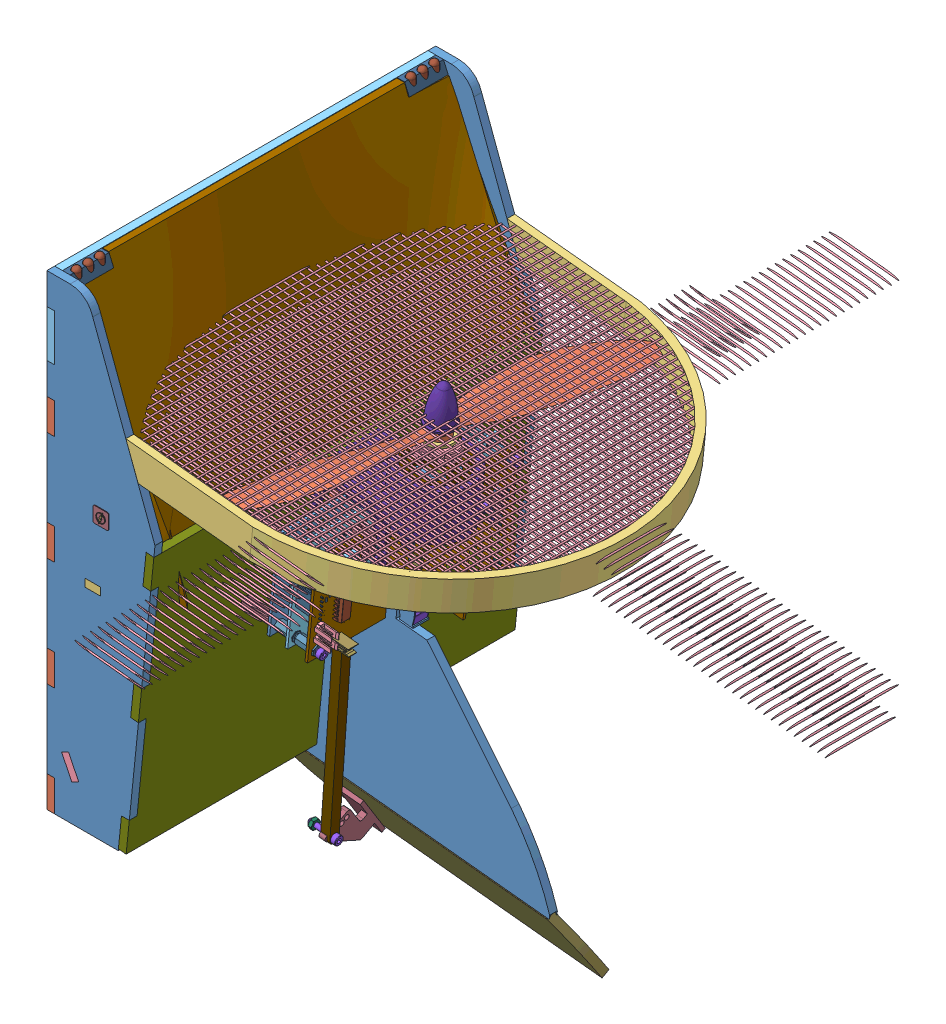
SolidWorks assembly AssTotaleSimu4, configuration Défaut. Lengths in mm. (continued)
Components (placement in the parent): (continued)
- AssStructSimu-1: AssStructSimu [Défaut] at (-125.7658 -1.8483 624.6548) x (1 0 0) z (0 0 -1) size (253.25 324.59 251.6) (continued)
  - AssCarte-1: AssCarte [Défaut] at (38.0121 147.1029 290.772) x (-0.101852 0.9948 0) z (0.9948 0.101852 0) size (66.52 130.57 98.72) (continued)
    - AssEntretoise-3: AssEntretoise [Défaut] at (-106.8199 -51.2976 37.1344) x (0 0 -1) z (1 0 0) size (58.24 7.29 7.81)
      - socket head cap screw 4762_din-1: socket head cap screw 4762_din [EN ISO 4762 M3 x 5 - 5N] at (-2.4967 0.5867 0) size (8 5.5 5.5)
      - hexagonal_spacer_MF_M3_H20_HEX5.5_FTD6_MTL6-1: hexagonal_spacer_MF_M3_H20_HEX5.5_FTD6_MTL6 [Défaut] at (48.3433 0.5867 0) x (0 0 1) z (-1 0 0) size (6.36 5.51 26)
      - hex nut style 1 gradeab_din-1: hex nut style 1 gradeab_din [Hexagon Nut ISO 4032 - M3 - W - N] at (53.3433 0.5867 0) x (0 0.943962 0.330053) z (-1 0 0) size (5.5 6.35 2.4)
      - hexagonal_spacer_MF_M3_H12_HEX5.5_FTD6_MTL6-2: hexagonal_spacer_MF_M3_H12_HEX5.5_FTD6_MTL6 [Défaut] at (27.0633 0.5867 0) x (0 0.248308 0.968681) z (-1 0 0) size (6.36 5.51 18)
      - hexagonal_spacer_MF_M3_H12_HEX5.5_FTD6_MTL6-3: hexagonal_spacer_MF_M3_H12_HEX5.5_FTD6_MTL6 [Défaut] at (13.7833 0.5867 0) x (0 0 1) z (-1 0 0) size (6.36 5.51 18)
    - AssEntretoise-4: AssEntretoise [Défaut] at (-106.8199 68.7024 37.1344) x (0 0 -1) z (1 0 0) size (58.24 7.29 7.81)
      - socket head cap screw 4762_din-1: socket head cap screw 4762_din [EN ISO 4762 M3 x 5 - 5N] at (-2.4967 0.5867 0) size (8 5.5 5.5)
      - hexagonal_spacer_MF_M3_H20_HEX5.5_FTD6_MTL6-1: hexagonal_spacer_MF_M3_H20_HEX5.5_FTD6_MTL6 [Défaut] at (48.3433 0.5867 0) x (0 0 1) z (-1 0 0) size (6.36 5.51 26)
      - hex nut style 1 gradeab_din-1: hex nut style 1 gradeab_din [Hexagon Nut ISO 4032 - M3 - W - N] at (53.3433 0.5867 0) x (0 0.943962 0.330053) z (-1 0 0) size (5.5 6.35 2.4)
      - hexagonal_spacer_MF_M3_H12_HEX5.5_FTD6_MTL6-2: hexagonal_spacer_MF_M3_H12_HEX5.5_FTD6_MTL6 [Défaut] at (27.0633 0.5867 0) x (0 0.248308 0.968681) z (-1 0 0) size (6.36 5.51 18)
      - hexagonal_spacer_MF_M3_H12_HEX5.5_FTD6_MTL6-3: hexagonal_spacer_MF_M3_H12_HEX5.5_FTD6_MTL6 [Défaut] at (13.7833 0.5867 0) x (0 0 1) z (-1 0 0) size (6.36 5.51 18)
    - AssMpu-1: AssMpu [Défaut] at (-150.6881 40.5798 29.6372) x (0.908747 0.417347 0) z (0 0 1) size (8 8 22.28)
      - hex nut style 1 gradeab_din-1: hex nut style 1 gradeab_din [Hexagon Nut ISO 4032 - M3 - W - N] at (0.2783 0.3227 1.2) size (5.5 6.35 2.4)
      - plain washer 6903 type ab_din-1: plain washer 6903 type ab_din [DIN 6903-A3] at (0.2783 0.3227 1.2) x (0 0 1) z (-1 0 0) size (1 8 8)
      - socket head cap screw 4762_din-1: socket head cap screw 4762_din [EN ISO 4762 M3 x 5 - 5N] at (0.2783 0.3227 19.76) x (0 0 -1) z (-0.852155 0.523289 0) size (8 5.5 5.5)
      - hexagonal_spacer_MF_M3_H12_HEX5.5_FTD6_MTL6-1: hexagonal_spacer_MF_M3_H12_HEX5.5_FTD6_MTL6 [Défaut] at (0.2783 0.3227 3.48) size (6.36 5.51 18)
    - AssMpu-2: AssMpu [Défaut] at (-130.3481 40.6665 29.6372) size (8 8 22.28)
      - hex nut style 1 gradeab_din-1: hex nut style 1 gradeab_din [Hexagon Nut ISO 4032 - M3 - W - N] at (0.2783 0.3227 1.2) size (5.5 6.35 2.4)
      - plain washer 6903 type ab_din-1: plain washer 6903 type ab_din [DIN 6903-A3] at (0.2783 0.3227 1.2) x (0 0 1) z (-1 0 0) size (1 8 8)
      - socket head cap screw 4762_din-1: socket head cap screw 4762_din [EN ISO 4762 M3 x 5 - 5N] at (0.2783 0.3227 19.76) x (0 0 -1) z (-0.852155 0.523289 0) size (8 5.5 5.5)
      - hexagonal_spacer_MF_M3_H12_HEX5.5_FTD6_MTL6-1: hexagonal_spacer_MF_M3_H12_HEX5.5_FTD6_MTL6 [Défaut] at (0.2783 0.3227 3.48) size (6.36 5.51 18)
    - AssCosse-1: AssCosse [Défaut] at (-142.6764 26.8797 71.168) x (0 -1 0) z (-0.344896 0 -0.938641) size (9.83 18.66 11.64)
      - socket head cap screw 4762_din-1: socket head cap screw 4762_din [EN ISO 4762 M3 x 6 - 6N] at (-5.1064 0.3659 0) size (9 5.5 5.5)
      - plain washer 6903 type ab_din-1: plain washer 6903 type ab_din [DIN 6903-A3] at (-2.1064 0.3659 0) size (1 8 8)
      - hex nut style 1 gradeab_din-2: hex nut style 1 gradeab_din [Hexagon Nut ISO 4032 - M3 - W - N] at (1.281 0.3659 0) x (0 0.924225 0.381849) z (-1 0 0) size (5.5 6.35 2.4)
      - 31880-1: 31880 [Default] at (0.4936 0.3659 0) x (0 0.344896 -0.938641) z (0 -0.938641 -0.344896) size (5.54 5 17.37)
    - AssCosse-2: AssCosse [Défaut] at (-142.6764 -2.9203 71.168) x (0 -1 0) z (-0.344896 0 -0.938641) size (9.83 18.66 11.64)
      - socket head cap screw 4762_din-1: socket head cap screw 4762_din [EN ISO 4762 M3 x 6 - 6N] at (-5.1064 0.3659 0) size (9 5.5 5.5)
      - plain washer 6903 type ab_din-1: plain washer 6903 type ab_din [DIN 6903-A3] at (-2.1064 0.3659 0) size (1 8 8)
      - hex nut style 1 gradeab_din-2: hex nut style 1 gradeab_din [Hexagon Nut ISO 4032 - M3 - W - N] at (1.281 0.3659 0) x (0 0.924225 0.381849) z (-1 0 0) size (5.5 6.35 2.4)
      - 31880-1: 31880 [Default] at (0.4936 0.3659 0) x (0 0.344896 -0.938641) z (0 -0.938641 -0.344896) size (5.54 5 17.37)
    - AssCosse-3: AssCosse [Défaut] at (-142.6764 12.0797 71.168) x (0 -1 0) z (-0.344896 0 -0.938641) size (9.83 18.66 11.64)
      - socket head cap screw 4762_din-1: socket head cap screw 4762_din [EN ISO 4762 M3 x 6 - 6N] at (-5.1064 0.3659 0) size (9 5.5 5.5)
      - plain washer 6903 type ab_din-1: plain washer 6903 type ab_din [DIN 6903-A3] at (-2.1064 0.3659 0) size (1 8 8)
      - hex nut style 1 gradeab_din-2: hex nut style 1 gradeab_din [Hexagon Nut ISO 4032 - M3 - W - N] at (1.281 0.3659 0) x (0 0.924225 0.381849) z (-1 0 0) size (5.5 6.35 2.4)
      - 31880-1: 31880 [Default] at (0.4936 0.3659 0) x (0 0.344896 -0.938641) z (0 -0.938641 -0.344896) size (5.54 5 17.37)
    - Terminal_QD_Female-1: Terminal_QD_Female [Default] at (-137.2199 31.5422 53.3942) x (0 1 0) z (-1 0 0) size (9.4 5.5 22.35)
    - Terminal_QD_Female-2: Terminal_QD_Female [Default] at (-137.3199 31.5422 36.2942) x (0 -1 0) z (-1 0 0) size (9.4 5.5 22.35)
    - Terminal_QD_Female-3: Terminal_QD_Female [Default] at (-137.2199 1.7422 53.3942) x (0 1 0) z (-1 0 0) size (9.4 5.5 22.35)
    - Terminal_QD_Female-4: Terminal_QD_Female [Default] at (-137.3199 1.7422 35.9942) x (0 1 0) z (-1 0 0) size (9.4 5.5 22.35)
    - Terminal_QD_Female-5: Terminal_QD_Female [Default] at (-137.3199 16.7422 35.9942) x (0 1 0) z (-1 0 0) size (9.4 5.5 22.35)
    - Terminal_QD_Female-6: Terminal_QD_Female [Default] at (-137.2199 16.7422 53.3942) x (0 1 0) z (-1 0 0) size (9.4 5.5 22.35)
- AssTige-1: AssTige [Défaut] at (-241.576 -121.7726 340.4233) x (-0.101791 -0.994204 -0.034587) z (0.9948 -0.101852 0) size (166.39 7.19 19)
  - tige_servo-1: tige_servo [Défaut] at (-106.2712 0.2685 162) size (165 6 6)
  - socket head cap screw 4762_din-2: socket head cap screw 4762_din [EN ISO 4762 M2 x 10 - 10N] at (-104.2712 3.2685 170) x (0 0 -1) z (0.923728 0.383049 0) size (12 3.8 3.8)
  - hex nut style 1 gradeab_din-1: hex nut style 1 gradeab_din [Hexagon Nut ISO 4032 - M3 - W - N] at (55.7288 3.2685 156) size (5.5 6.35 2.4)
  - hex nut style 1 gradeab_din-2: hex nut style 1 gradeab_din [Hexagon Nut ISO 4032 - M2 - W - N] at (-104.2712 3.2685 160) x (0.904801 0.425836 0) z (0 0 1) size (4 4.62 1.6)
  - socket head cap screw 4762_din-3: socket head cap screw 4762_din [EN ISO 4762 M3 x 16 - 16N] at (55.7288 3.2685 171) x (0 0 -1) z (0.923728 0.383049 0) size (19 5.5 5.5)
- AssGoPro-1: AssGoPro [Défaut] at (-119.9926 15.1708 318.2917) x (0 0 -1) z (-0.119031 -0.99289 0) size (64.3 52.3 34.42)
  - GoPRo Frame for LCD Screen-1: GoPRo Frame for LCD Screen [Défaut] at (-2.6935 10.9558 5.5635) size (64.3 59.3 34.42)
    - GoProFrame MJM-1: GoProFrame MJM [Défaut] at (-3.6084 -1.6692 52.45) size (64.3 59.3 23.5)
    - GoPro Hero 3 Front Panel-1: GoPro Hero 3 Front Panel [Défaut] at (-3.6084 -1.6692 55.7) x (-1 0 0) z (0 0 -1) size (59.25 41.2 1.9)
    - GoPro Hero 3 Screen-1: GoPro Hero 3 Screen [Défaut] at (12.7166 3.9308 54.9) size (15 18 1)
    - GoPro Hero 3 Mode Button-1: GoPro Hero 3 Mode Button [Défaut] at (13.4166 -12.4692 54.95) x (-1 0 0) z (0 0 -1) size (11.97 12.11 3.03)
    - GoPro Hero 3 LED Cover-1: GoPro Hero 3 LED Cover [Défaut] at (3.1166 -9.3192 54.85) x (-0.999988 0.004848 0) z (0 0 -1) size (5 5 1.4)
    - GoPro Hero 3 LED Cover-2: GoPro Hero 3 LED Cover [Défaut] at (3.1166 -16.0692 54.85) x (-0.999988 0.004848 0) z (0 0 -1) size (5 5 1.4)
    - GoPro Hero 3 Housing-1: GoPro Hero 3 Housing [Défaut] at (-3.6084 -1.6692 55.7) size (59.37 41.3 29.84)
    - GoPro Hero 3 Lens-1: GoPro Hero 3 Lens [Défaut] at (-18.9334 5.6308 47.35) x (-0.380542 -0.924764 0) z (0 0 -1) size (13.71 15.7 7.94)
    - GoPro Hero 3 Indicator Cover-1: GoPro Hero 3 Indicator Cover [Défaut] at (-25.5834 -22.2692 69.9) x (-0.997412 0 -0.0719) z (0 1 0) size (3 3 2)
    - GoPro Hero 3 Indicator Cover-2: GoPro Hero 3 Indicator Cover [Défaut] at (-28.8834 12.2308 73) x (-0.999992 0.004018 0) z (0 0 1) size (3 3 2)
    - GoPro Hero 3 Indicator Cover-3: GoPro Hero 3 Indicator Cover [Défaut] at (20.6666 16.9308 58.4) x (-0.997739 0 -0.067212) z (0 1 0) size (3 3 2)
    - slot-1: slot [Défaut] at (-24.7434 -9.7363 65.05) x (0 1 0) z (0 0 -1) size (16 15.02 2.44)
    - GoPro Hero 3 HDMI pin-1: GoPro Hero 3 HDMI pin [Défaut] at (-26.982 2.9815 24.7172) x (0.105491 0.98175 -0.158237) z (-0.992872 0.095109 -0.071829) size (3.29 0.86 3.28)
  - support1-2: support1 [Défaut] at (-1.3019 -18.8633 67.0135) x (0 0 1) z (-1 0 0) size (5 5 10)
- AssGouv-1: AssGouv [Défaut] at (-43.2668 -298.2106 479.8345) x (0.9948 -0.101852 0) z (0.055947 0.546439 -0.835628) size (200.18 52.5 43.47)
  - P10_1-1: P10_1 [Défaut] at (-108.1667 -19.4144 197.6829) size (200.18 50.13 5)
  - attache_pale-1: attache_pale [Défaut] at (-49.1667 8.0856 190.1829) x (0 0 -1) z (-1 0 0) size (43.47 35 14)
- Parallax-Servo-Horn-1: Parallax-Servo-Horn [Défaut] at (-69.3162 -29.8353 324.5606) x (0.09792 0.956393 0.27518) z (0.9948 -0.101852 0) size (38.81 38.81 6.17)
- NTM_35-36_engine_assembly-1: NTM_35-36_engine_assembly [Défaut] at (-24.3523 26.8781 325.7101) x (0.9948 -0.101852 0) z (0 0 1) size (60.56 77.2 246.41)
  - engine_base-1: engine_base [Défaut] at (-1.8719 -19.5526 -1.1165) x (0 1 0) z (0 0 1) size (6.8 35 35)
  - engine_bearing-1: engine_bearing [Défaut] at origin size (10 4 10)
  - Propeller_cone-1: Propeller_cone [Défaut] at (-1.8719 33.6474 -4.1165) x (1 0 0) z (0 1 0) size (17.6 17.6 24)
  - engine_bearing-2: engine_bearing [Défaut] at (0 22.8 0) size (10 4 10)
  - NTM_35-36_enginebody-1: NTM_35-36_enginebody [Défaut] at (-1.8719 -12.7526 -1.1165) size (35 31.7 35)
  - Stator-1: Stator [Défaut] at origin size (27.75 22.36 27.94)
  - propellers_10x4-1: propellers_10x4 [Défaut] at (-6.8719 27.4474 -4.9165) size (60.56 10.53 246.41)
  - propeller_washer-1: propeller_washer [Défaut] at (-1.8719 24.4474 -1.1165) x (0 1 0) z (0 0 1) size (2.5 18 18)
  - Propeller_adaptor-1: Propeller_adaptor [Défaut] at (2.1948 17.1101 -3.713) size (23.46 32.5 25)
Mates (geometry in assembly coordinates):
- Coaxiale1: concentric aligned: cylinder of AssStructSimu-1/AssToitMot-1/AssToit-1/P12-1 through (-27.6967 12.5918 324.5936) axis (-0.101852 -0.9948 0) radius 17.5; cylinder of NTM_35-36_engine_assembly-1/NTM_35-36_enginebody-1 through (-25.2217 36.7654 324.5936) axis (-0.101852 -0.9948 0) radius 17.5
- Coïncidente1: coincident anti-aligned: plane of AssStructSimu-1/AssToitMot-1/AssToit-1/P12-1 through (-28.206 7.6178 324.5936) normal (0.101852 0.9948 0); plane of NTM_35-36_engine_assembly-1/engine_bearing-1 through (-28.206 7.6178 324.5936) normal (-0.101852 -0.9948 0)
- Coaxiale2: concentric aligned: cylinder of AssStructSimu-1/AssToitMot-1/AssToit-1/P10_2-1 through (49.7135 -178.7878 324.5936) axis (-0.9948 0.101852 0) radius 2.5; cylinder of AssGouv-1/P10_1-1 through (-94.0351 -164.0702 324.5936) axis (-0.9948 0.101852 0) radius 2.5
- Coïncidente2: coincident aligned: plane of AssStructSimu-1/AssToitMot-1/AssToit-1/P10_2-1 through (-137.5516 -157.1017 322.0936) normal (-0.9948 0.101852 0); plane of AssGouv-1/P10_1-1 through (-137.8791 -160.3008 321.1312) normal (-0.9948 0.101852 0)
- Coaxiale3: concentric aligned: cylinder of AssTige-1/socket head cap screw 4762_din-3 through (-45.5416 -197.7164 335.2292) axis (0.9948 -0.101852 0) radius 1.5; cylinder of AssGouv-1/attache_pale-1 through (-85.9983 -193.5742 335.2292) axis (0.9948 -0.101852 0) radius 1.5
- Coaxiale4: concentric aligned: cylinder of AssStructSimu-1/AssToitMot-1/Parallax-Servo_DUMMY-1 through (-70.6554 -29.6982 324.5606) axis (-0.9948 0.101852 0) radius 2.9845; cylinder of Parallax-Servo-Horn-1 through (-70.6554 -29.6982 324.5606) axis (-0.9948 0.101852 0) radius 2.9845
- Coïncidente3: coincident anti-aligned: plane of AssStructSimu-1/AssToitMot-1/Parallax-Servo_DUMMY-1 through (-74.8246 -29.2713 324.5606) normal (0.9948 -0.101852 0); plane of Parallax-Servo-Horn-1 through (-74.8246 -29.2713 324.5606) normal (-0.9948 0.101852 0)
- Coaxiale5: concentric anti-aligned: cylinder of AssTige-1/socket head cap screw 4762_din-2 through (-30.2498 -38.5418 340.7631) axis (0.9948 -0.101852 0) radius 1; cylinder of Parallax-Servo-Horn-1 through (-69.7931 -34.4932 340.7631) axis (-0.9948 0.101852 0) radius 0.635
- Coïncidente4: coincident anti-aligned: plane of AssTige-1/tige_servo-1 through (-69.6001 -32.608 343.8305) normal (-0.9948 0.101852 0); plane of Parallax-Servo-Horn-1 through (-68.8748 -25.5237 332.3708) normal (0.9948 -0.101852 0)
- Coaxiale6: concentric aligned: cylinder of AssStructSimu-1/AssBase-1/socket head cap screw 4762_din-7 through (-144.5139 -51.9008 369.3436) axis (0 0 1) radius 1.5; cylinder of AssGoPro-1/support1-2 through (-144.5139 -51.9008 319.5936) axis (0 0 1) radius 1.5
- Coïncidente5: coincident anti-aligned: plane of AssStructSimu-1/AssBase-1/support2-1 through (-141.9706 -54.3568 329.5936) normal (0 0 -1); plane of AssGoPro-1/support1-2 through (-146.6985 -49.121 329.5936) normal (0 0 1)
